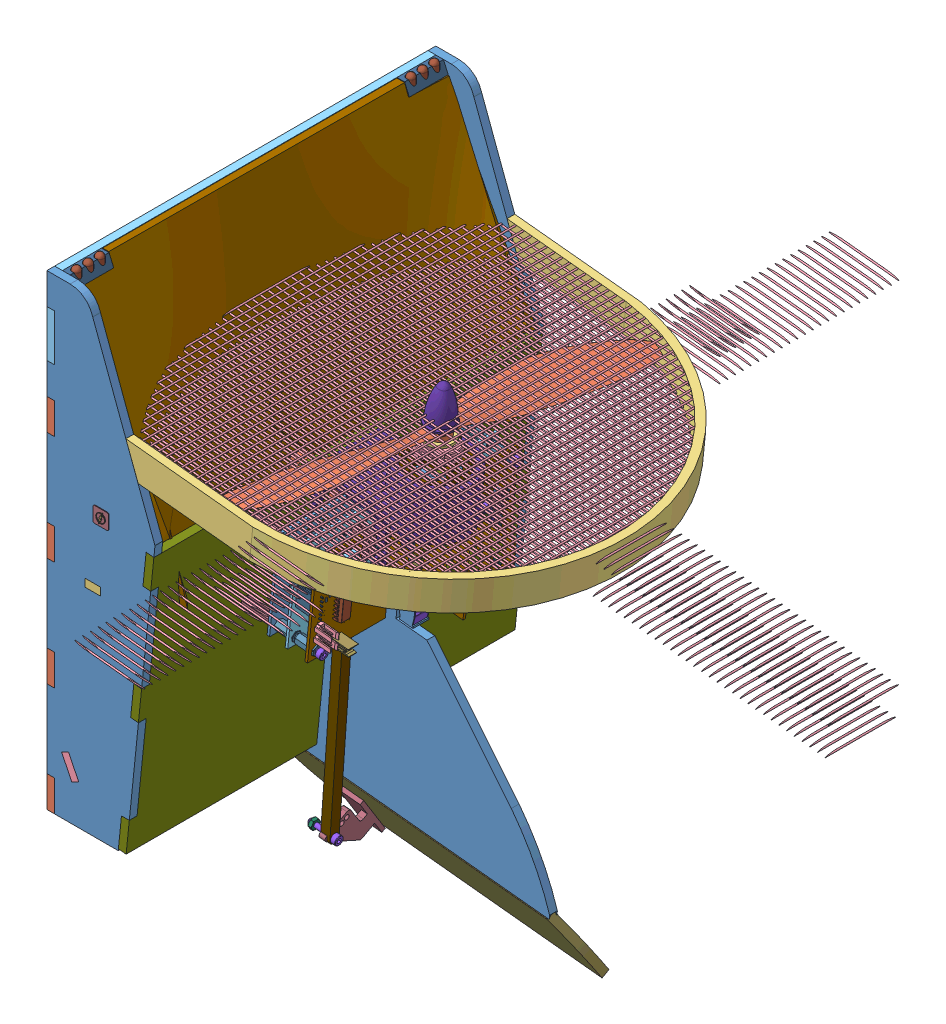
SolidWorks assembly AssTotaleSimu3, configuration Défaut. Lengths in mm. (continued)
Components (placement in the parent): (continued)
- AssStructSimu-1: AssStructSimu [Défaut] at (-125.7658 -1.8483 624.6548) x (1 0 0) z (0 0 -1) size (253.25 324.59 251.6) (continued)
  - AssProtec-1: AssProtec [Défaut] at (86.6746 190.4649 284.6351) x (0 0 -1) z (0.101852 -0.9948 0) size (250 237.46 20) (continued)
    - AssGrillage-2: AssGrillage [Défaut] at (339.6086 -132.5428 241.6839) x (0 0 1) z (-1 0 0) size (2.02 237.05 250) (continued)
      - barreau-208: barreau [Défaut] at (-0.1839 -1.5314 233.7823) x (0.998922 0 0.04641) z (0 1 0) size (1 1 400)
      - barreau-209: barreau [Défaut] at (-0.1839 -1.5314 228.7823) x (0.998922 0 0.04641) z (0 1 0) size (1 1 400)
      - barreau-210: barreau [Défaut] at (-0.1839 -1.5314 223.7823) x (0.998922 0 0.04641) z (0 1 0) size (1 1 400)
      - barreau-211: barreau [Défaut] at (-0.1839 -1.5314 218.7823) x (0.998922 0 0.04641) z (0 1 0) size (1 1 400)
      - barreau-212: barreau [Défaut] at (-0.1839 -1.5314 213.7823) x (0.998922 0 0.04641) z (0 1 0) size (1 1 400)
      - barreau-213: barreau [Défaut] at (-0.1839 -1.5314 208.7823) x (0.998922 0 0.04641) z (0 1 0) size (1 1 400)
      - barreau-214: barreau [Défaut] at (-0.1839 -1.5314 203.7823) x (0.998922 0 0.04641) z (0 1 0) size (1 1 400)
  - AssCarte-1: AssCarte [Défaut] at (38.0121 147.1029 290.772) x (-0.101852 0.9948 0) z (0.9948 0.101852 0) size (66.52 130.57 98.72)
    - carte_onduleur_v3-1: carte_onduleur_v3 [Défaut] at (-131.8199 12.0892 20.7912) size (66.52 130.57 82.34)
      - Layer_1-1: Layer_1 [Défaut] at origin size (60 130 1.61)
      - BTN-1: BTN [Défaut] at (-25.5 7.4 0.803) x (0 -1 0) z (0 0 1) size (6.76 3.64 4.37)
        - Open CASCADE STEP translator 6.8 1.2.1-1: Open CASCADE STEP translator 6.8 1.2.1 [Défaut] at origin size (6.76 3.64 4.37)
          - Body_1-1: Body_1 [Défaut] at (-0.5 -2 0) size (6.76 3.64 4.37)
            - =_[0_1_1_3]-1: =_[0_1_1_3] [Défaut] at origin size (6 3.64 4.37)
            - =_[0_1_1_4]-1: =_[0_1_1_4] [Défaut] at origin size (0.38 1 0.67)
            - =_[0_1_1_5]-1: =_[0_1_1_5] [Défaut] at origin size (0.38 1 0.67)
      - CON_IO1-1: CON_IO1 [Défaut] at (-11.3 12.1 0.803) x (0 -1 0) z (0 0 1) size (13 30 57.5)
        - Open CASCADE STEP translator 6.8 1.3.1-1: Open CASCADE STEP translator 6.8 1.3.1 [Défaut] at origin size (13 30 57.5)
          - Body_1_2-1: Body_1_2 [Défaut] at (-3 -15 8) x (0 -1 0) z (-1 0 0) size (30 57.5 13)
            - 1-1: 1 [Défaut] at origin size (30 50 1.61)
            - 10-1: 10 [Défaut] at (-14.395 31.0465 0.803) x (-1 0 0) z (0 0 1) size (5.59 6.35 1.11)
              - =_[0_1_1_4]-1: =_[0_1_1_4] [Défaut] at origin size (5.59 6.35 1.11)
                - 11-1: 11 [Défaut] at (2 3.3 0) x (-1 0 0) z (0 0 1) size (5.59 6.35 1.11)
                  - =_[0_1_1_3]_2-1: =_[0_1_1_3]_2 [Défaut] at origin size (0.44 0.55 0.36)
                  - =_[0_1_1_4]_2-1: =_[0_1_1_4]_2 [Défaut] at origin size (5.59 4.15 0.36)
                  - =_[0_1_1_5]_2-1: =_[0_1_1_5]_2 [Défaut] at origin size (5.35 6.1 1.1)
                  - =_[0_1_1_6]-1: =_[0_1_1_6] [Défaut] at origin size (0.44 0.55 0.36)
                  - =_[0_1_1_7]-1: =_[0_1_1_7] [Défaut] at origin size (0.44 0.55 0.36)
                  - =_[0_1_1_8]-1: =_[0_1_1_8] [Défaut] at origin size (0.44 0.55 0.36)
            - 13-1: 13 [Défaut] at (-12.62 16.6 -0.803) x (-1 0 0) z (0 0 -1) size (5.59 6.35 1.11)
              - =_[0_1_1_13]-1: =_[0_1_1_13] [Défaut] at origin size (5.59 6.35 1.11)
                - 11-1: 11 [Défaut] at (2 3.3 0) x (-1 0 0) z (0 0 1) size (5.59 6.35 1.11)
                  - =_[0_1_1_3]_2-1: =_[0_1_1_3]_2 [Défaut] at origin size (0.44 0.55 0.36)
                  - =_[0_1_1_4]_2-1: =_[0_1_1_4]_2 [Défaut] at origin size (5.59 4.15 0.36)
                  - =_[0_1_1_5]_2-1: =_[0_1_1_5]_2 [Défaut] at origin size (5.35 6.1 1.1)
                  - =_[0_1_1_6]-1: =_[0_1_1_6] [Défaut] at origin size (0.44 0.55 0.36)
                  - =_[0_1_1_7]-1: =_[0_1_1_7] [Défaut] at origin size (0.44 0.55 0.36)
                  - =_[0_1_1_8]-1: =_[0_1_1_8] [Défaut] at origin size (0.44 0.55 0.36)
            - 16-1: 16 [Défaut] at (-4.2 24.2 0.803) x (-1 0 0) z (0 0 1) size (12.8 0.5 13)
              - =_[0_1_1_15]-1: =_[0_1_1_15] [Défaut] at origin size (12.8 0.5 13)
                - 17-1: 17 [Défaut] at (2.7 0 0) x (1 0 0) z (0 -1 0) size (12.8 13 0.5)
            - 19-1: 19 [Défaut] at (-4.1 6.8 0.803) x (-1 0 0) z (0 0 1) size (12.8 0.5 13)
              - =_[0_1_1_18]-1: =_[0_1_1_18] [Défaut] at origin size (12.8 0.5 13)
                - 17-1: 17 [Défaut] at (2.7 0 0) x (1 0 0) z (0 -1 0) size (12.8 13 0.5)
            - 24-1: 24 [Défaut] at (-8.1 16.5 -0.803) x (0 1 0) z (0 0 -1) size (7.75 5.13 1.17)
              - =_[0_1_1_20]-1: =_[0_1_1_20] [Défaut] at origin size (7.75 5.13 1.17)
                - 20-1: 20 [Défaut] at origin size (7.59 5.13 1.07)
                - 21-1: 21 [Défaut] at (-14.478 0 0) x (-1 0 0) z (0 0 1) size (0.76 5.08 1.17)
                - 22-1: 22 [Défaut] at origin size (0.76 5.08 1.17)
            - 35-1: 35 [Défaut] at (-25.3 25.5 0.803) x (0 -1 0) z (0 0 1) size (6.05 5.2 1.7)
              - =_[0_1_1_25]-1: =_[0_1_1_25] [Défaut] at origin size (6.05 5.2 1.7)
                - 25-1: 25 [Défaut] at origin size (4.3 5.2 1.53)
                - 26-1: 26 [Défaut] at origin size (0.88 0.51 1.06)
                - 27-1: 27 [Défaut] at origin size (0.88 0.51 1.06)
                - 28-1: 28 [Défaut] at origin size (0.88 0.51 1.06)
                - 29-1: 29 [Défaut] at origin size (0.88 0.51 1.06)
                - 30-1: 30 [Défaut] at (11.6 -5.08 0) x (-1 0 0) z (0 0 1) size (0.87 0.51 1.06)
                - 31-1: 31 [Défaut] at (11.6 -2.54 0) x (-1 0 0) z (0 0 1) size (0.87 0.51 1.06)
                - 32-1: 32 [Défaut] at (11.6 0 0) x (-1 0 0) z (0 0 1) size (0.87 0.51 1.06)
                - 33-1: 33 [Défaut] at (11.6 2.54 0) x (-1 0 0) z (0 0 1) size (0.87 0.51 1.06)
            - 40-1: 40 [Défaut] at (-27.6 27.2 0.803) size (2.34 1.04 0.5)
              - =_[0_1_1_36]-1: =_[0_1_1_36] [Défaut] at origin size (2.34 1.04 0.5)
                - 36-1: 36 [Défaut] at origin size (2.29 1.04 0.43)
                - 37-1: 37 [Défaut] at (0.3048 0 0) x (-1 0 0) z (0 0 1) size (0.51 1.02 0.5)
                - 38-1: 38 [Défaut] at origin size (0.51 1.02 0.5)
            - 42-1: 42 [Défaut] at (-22.1 21.6 0.803) x (0 1 0) z (0 0 1) size (2.34 1.04 0.5)
              - =_[0_1_1_36]-1: =_[0_1_1_36] [Défaut] at origin size (2.34 1.04 0.5)
                - 36-1: 36 [Défaut] at origin size (2.29 1.04 0.43)
                - 37-1: 37 [Défaut] at (0.3048 0 0) x (-1 0 0) z (0 0 1) size (0.51 1.02 0.5)
                - 38-1: 38 [Défaut] at origin size (0.51 1.02 0.5)
            - 47-1: 47 [Défaut] at (-14.7664 14.5 -0.803) x (-1 0 0) z (0 0 -1) size (2.34 1.04 0.5)
              - =_[0_1_1_42]-1: =_[0_1_1_42] [Défaut] at origin size (2.34 1.04 0.5)
                - 43-1: 43 [Défaut] at origin size (2.29 1.04 0.43)
                - 44-1: 44 [Défaut] at (0.3048 0 0) x (-1 0 0) z (0 0 1) size (0.51 1.02 0.5)
                - 45-1: 45 [Défaut] at origin size (0.51 1.02 0.5)
            - 57-1: 57 [Défaut] at (-15.3 2.7 -0.803) x (0 -1 0) z (0 0 -1) size (10.36 15.24 6.14)
              - =_[0_1_1_47]-1: =_[0_1_1_47] [Défaut] at origin size (10.36 15.24 6.14)
                - 55-1: 55 [Défaut] at (1.8 -1.2 3) x (1 0 0) z (0 1 0) size (10.36 6.14 15.24)
                  - 54-1: 54 [Défaut] at origin size (10.36 6.14 7.62)
                    - 52-1: 52 [Défaut] at origin size (10.36 6.14 2.54)
                      - 48-1: 48 [Défaut] at origin size (8.4 2.54 2.54)
                      - 49-1: 49 [Défaut] at (-0.0461 1.2682 1.27) x (0 0 -1) z (0.999998 -0.002105 0) size (1.95 5.07 7.58)
                    - 52-2: 52 [Défaut] at (0 0 -2.54) size (10.36 6.14 2.54)
                      - 48-1: 48 [Défaut] at origin size (8.4 2.54 2.54)
                      - 49-1: 49 [Défaut] at (-0.0461 1.2682 1.27) x (0 0 -1) z (0.999998 -0.002105 0) size (1.95 5.07 7.58)
                    - 52-3: 52 [Défaut] at (0 0 -5.08) size (10.36 6.14 2.54)
                      - 48-1: 48 [Défaut] at origin size (8.4 2.54 2.54)
                      - 49-1: 49 [Défaut] at (-0.0461 1.2682 1.27) x (0 0 -1) z (0.999998 -0.002105 0) size (1.95 5.07 7.58)
                  - 54-2: 54 [Défaut] at (0 0 -7.62) size (10.36 6.14 7.62)
                    - 52-1: 52 [Défaut] at origin size (10.36 6.14 2.54)
                      - 48-1: 48 [Défaut] at origin size (8.4 2.54 2.54)
                      - 49-1: 49 [Défaut] at (-0.0461 1.2682 1.27) x (0 0 -1) z (0.999998 -0.002105 0) size (1.95 5.07 7.58)
                    - 52-2: 52 [Défaut] at (0 0 -2.54) size (10.36 6.14 2.54)
                      - 48-1: 48 [Défaut] at origin size (8.4 2.54 2.54)
                      - 49-1: 49 [Défaut] at (-0.0461 1.2682 1.27) x (0 0 -1) z (0.999998 -0.002105 0) size (1.95 5.07 7.58)
                    - 52-3: 52 [Défaut] at (0 0 -5.08) size (10.36 6.14 2.54)
                      - 48-1: 48 [Défaut] at origin size (8.4 2.54 2.54)
                      - 49-1: 49 [Défaut] at (-0.0461 1.2682 1.27) x (0 0 -1) z (0.999998 -0.002105 0) size (1.95 5.07 7.58)
            - 59-1: 59 [Défaut] at (-26.5 31 0.803) x (0 -1 0) z (0 0 1) size (2.34 1.04 0.5)
              - =_[0_1_1_42]-1: =_[0_1_1_42] [Défaut] at origin size (2.34 1.04 0.5)
                - 43-1: 43 [Défaut] at origin size (2.29 1.04 0.43)
                - 44-1: 44 [Défaut] at (0.3048 0 0) x (-1 0 0) z (0 0 1) size (0.51 1.02 0.5)
                - 45-1: 45 [Défaut] at origin size (0.51 1.02 0.5)
            - 61-1: 61 [Défaut] at (-21.6 17.8 0.803) x (-1 0 0) z (0 0 1) size (2.34 1.04 0.5)
              - =_[0_1_1_42]-1: =_[0_1_1_42] [Défaut] at origin size (2.34 1.04 0.5)
                - 43-1: 43 [Défaut] at origin size (2.29 1.04 0.43)
                - 44-1: 44 [Défaut] at (0.3048 0 0) x (-1 0 0) z (0 0 1) size (0.51 1.02 0.5)
                - 45-1: 45 [Défaut] at origin size (0.51 1.02 0.5)
            - 74-1: 74 [Défaut] at (-4.9 41.8 0.803) x (0 -1 0) z (0 0 1) size (6 4.9 1.75)
              - =_[0_1_1_56]-1: =_[0_1_1_56] [Défaut] at origin size (6 4.9 1.75)
                - 72-1: 72 [Défaut] at origin size (6 4.9 1.75)
                  - =_[0_1_1_2]-1: =_[0_1_1_2] [Défaut] at origin size (3.9 4.9 1.57)
                  - =_[0_1_1_3]-1: =_[0_1_1_3] [Défaut] at origin size (6 4.22 1)
                    - =_[0_1_1_60]-1: =_[0_1_1_60] [Défaut] at origin size (1.05 0.41 1)
                    - =_[0_1_1_61]-1: =_[0_1_1_61] [Défaut] at origin size (1.05 0.41 1)
                    - =_[0_1_1_62]-1: =_[0_1_1_62] [Défaut] at origin size (1.05 0.41 1)
                    - =_[0_1_1_63]-1: =_[0_1_1_63] [Défaut] at origin size (1.05 0.41 1)
                    - =_[0_1_1_64]-1: =_[0_1_1_64] [Défaut] at origin size (1.05 0.41 1)
                    - =_[0_1_1_65]-1: =_[0_1_1_65] [Défaut] at origin size (1.05 0.41 1)
                    - =_[0_1_1_66]-1: =_[0_1_1_66] [Défaut] at origin size (1.05 0.41 1)
                    - =_[0_1_1_67]-1: =_[0_1_1_67] [Défaut] at origin size (1.05 0.41 1)
            - 76-1: 76 [Défaut] at (-8.5 40.5664 0.803) x (0 1 0) z (0 0 1) size (2.34 1.04 0.5)
              - =_[0_1_1_42]-1: =_[0_1_1_42] [Défaut] at origin size (2.34 1.04 0.5)
                - 43-1: 43 [Défaut] at origin size (2.29 1.04 0.43)
                - 44-1: 44 [Défaut] at (0.3048 0 0) x (-1 0 0) z (0 0 1) size (0.51 1.02 0.5)
                - 45-1: 45 [Défaut] at origin size (0.51 1.02 0.5)
            - 78-1: 78 [Défaut] at (-5.9 46.4 0.803) x (-1 0 0) z (0 0 1) size (2.34 1.04 0.5)
              - =_[0_1_1_42]-1: =_[0_1_1_42] [Défaut] at origin size (2.34 1.04 0.5)
                - 43-1: 43 [Défaut] at origin size (2.29 1.04 0.43)
                - 44-1: 44 [Défaut] at (0.3048 0 0) x (-1 0 0) z (0 0 1) size (0.51 1.02 0.5)
                - 45-1: 45 [Défaut] at origin size (0.51 1.02 0.5)
            - 80-1: 80 [Défaut] at (-7 48.1 0.803) size (2.34 1.04 0.5)
              - =_[0_1_1_42]-1: =_[0_1_1_42] [Défaut] at origin size (2.34 1.04 0.5)
                - 43-1: 43 [Défaut] at origin size (2.29 1.04 0.43)
                - 44-1: 44 [Défaut] at (0.3048 0 0) x (-1 0 0) z (0 0 1) size (0.51 1.02 0.5)
                - 45-1: 45 [Défaut] at origin size (0.51 1.02 0.5)
            - 82-1: 82 [Défaut] at (-6 37.1 0.803) size (2.34 1.04 0.5)
              - =_[0_1_1_42]-1: =_[0_1_1_42] [Défaut] at origin size (2.34 1.04 0.5)
                - 43-1: 43 [Défaut] at origin size (2.29 1.04 0.43)
                - 44-1: 44 [Défaut] at (0.3048 0 0) x (-1 0 0) z (0 0 1) size (0.51 1.02 0.5)
                - 45-1: 45 [Défaut] at origin size (0.51 1.02 0.5)
      - CON_IO2-1: CON_IO2 [Défaut] at (-11.3 -2.7 0.803) x (0 -1 0) z (0 0 1) size (13 30 57.5)
        - Open CASCADE STEP translator 6.8 1.4.1-1: Open CASCADE STEP translator 6.8 1.4.1 [Défaut] at origin size (13 30 57.5)
          - Body_1_2-1: Body_1_2 [Défaut] at (-3 -15 8) x (0 -1 0) z (-1 0 0) size (30 57.5 13)
            - 1-1: 1 [Défaut] at origin size (30 50 1.61)
            - 10-1: 10 [Défaut] at (-14.395 31.0465 0.803) x (-1 0 0) z (0 0 1) size (5.59 6.35 1.11)
              - =_[0_1_1_4]-1: =_[0_1_1_4] [Défaut] at origin size (5.59 6.35 1.11)
                - 11-1: 11 [Défaut] at (2 3.3 0) x (-1 0 0) z (0 0 1) size (5.59 6.35 1.11)
                  - =_[0_1_1_3]_2-1: =_[0_1_1_3]_2 [Défaut] at origin size (0.44 0.55 0.36)
                  - =_[0_1_1_4]_2-1: =_[0_1_1_4]_2 [Défaut] at origin size (5.59 4.15 0.36)
                  - =_[0_1_1_5]_2-1: =_[0_1_1_5]_2 [Défaut] at origin size (5.35 6.1 1.1)
                  - =_[0_1_1_6]-1: =_[0_1_1_6] [Défaut] at origin size (0.44 0.55 0.36)
                  - =_[0_1_1_7]-1: =_[0_1_1_7] [Défaut] at origin size (0.44 0.55 0.36)
                  - =_[0_1_1_8]-1: =_[0_1_1_8] [Défaut] at origin size (0.44 0.55 0.36)
            - 13-1: 13 [Défaut] at (-12.62 16.6 -0.803) x (-1 0 0) z (0 0 -1) size (5.59 6.35 1.11)
              - =_[0_1_1_13]-1: =_[0_1_1_13] [Défaut] at origin size (5.59 6.35 1.11)
                - 11-1: 11 [Défaut] at (2 3.3 0) x (-1 0 0) z (0 0 1) size (5.59 6.35 1.11)
                  - =_[0_1_1_3]_2-1: =_[0_1_1_3]_2 [Défaut] at origin size (0.44 0.55 0.36)
                  - =_[0_1_1_4]_2-1: =_[0_1_1_4]_2 [Défaut] at origin size (5.59 4.15 0.36)
                  - =_[0_1_1_5]_2-1: =_[0_1_1_5]_2 [Défaut] at origin size (5.35 6.1 1.1)
                  - =_[0_1_1_6]-1: =_[0_1_1_6] [Défaut] at origin size (0.44 0.55 0.36)
                  - =_[0_1_1_7]-1: =_[0_1_1_7] [Défaut] at origin size (0.44 0.55 0.36)
                  - =_[0_1_1_8]-1: =_[0_1_1_8] [Défaut] at origin size (0.44 0.55 0.36)
            - 16-1: 16 [Défaut] at (-4.2 24.2 0.803) x (-1 0 0) z (0 0 1) size (12.8 0.5 13)
              - =_[0_1_1_15]-1: =_[0_1_1_15] [Défaut] at origin size (12.8 0.5 13)
                - 17-1: 17 [Défaut] at (2.7 0 0) x (1 0 0) z (0 -1 0) size (12.8 13 0.5)
            - 19-1: 19 [Défaut] at (-4.1 6.8 0.803) x (-1 0 0) z (0 0 1) size (12.8 0.5 13)
              - =_[0_1_1_18]-1: =_[0_1_1_18] [Défaut] at origin size (12.8 0.5 13)
                - 17-1: 17 [Défaut] at (2.7 0 0) x (1 0 0) z (0 -1 0) size (12.8 13 0.5)
            - 24-1: 24 [Défaut] at (-8.1 16.5 -0.803) x (0 1 0) z (0 0 -1) size (7.75 5.13 1.17)
              - =_[0_1_1_20]-1: =_[0_1_1_20] [Défaut] at origin size (7.75 5.13 1.17)
                - 20-1: 20 [Défaut] at origin size (7.59 5.13 1.07)
                - 21-1: 21 [Défaut] at (-14.478 0 0) x (-1 0 0) z (0 0 1) size (0.76 5.08 1.17)
                - 22-1: 22 [Défaut] at origin size (0.76 5.08 1.17)
            - 35-1: 35 [Défaut] at (-25.3 25.5 0.803) x (0 -1 0) z (0 0 1) size (6.05 5.2 1.7)
              - =_[0_1_1_25]-1: =_[0_1_1_25] [Défaut] at origin size (6.05 5.2 1.7)
                - 25-1: 25 [Défaut] at origin size (4.3 5.2 1.53)
                - 26-1: 26 [Défaut] at origin size (0.88 0.51 1.06)
                - 27-1: 27 [Défaut] at origin size (0.88 0.51 1.06)
                - 28-1: 28 [Défaut] at origin size (0.88 0.51 1.06)
                - 29-1: 29 [Défaut] at origin size (0.88 0.51 1.06)
                - 30-1: 30 [Défaut] at (11.6 -5.08 0) x (-1 0 0) z (0 0 1) size (0.87 0.51 1.06)
                - 31-1: 31 [Défaut] at (11.6 -2.54 0) x (-1 0 0) z (0 0 1) size (0.87 0.51 1.06)
                - 32-1: 32 [Défaut] at (11.6 0 0) x (-1 0 0) z (0 0 1) size (0.87 0.51 1.06)
                - 33-1: 33 [Défaut] at (11.6 2.54 0) x (-1 0 0) z (0 0 1) size (0.87 0.51 1.06)
            - 40-1: 40 [Défaut] at (-27.6 27.2 0.803) size (2.34 1.04 0.5)
              - =_[0_1_1_36]-1: =_[0_1_1_36] [Défaut] at origin size (2.34 1.04 0.5)
                - 36-1: 36 [Défaut] at origin size (2.29 1.04 0.43)
                - 37-1: 37 [Défaut] at (0.3048 0 0) x (-1 0 0) z (0 0 1) size (0.51 1.02 0.5)
                - 38-1: 38 [Défaut] at origin size (0.51 1.02 0.5)
            - 42-1: 42 [Défaut] at (-22.1 21.6 0.803) x (0 1 0) z (0 0 1) size (2.34 1.04 0.5)
              - =_[0_1_1_36]-1: =_[0_1_1_36] [Défaut] at origin size (2.34 1.04 0.5)
                - 36-1: 36 [Défaut] at origin size (2.29 1.04 0.43)
                - 37-1: 37 [Défaut] at (0.3048 0 0) x (-1 0 0) z (0 0 1) size (0.51 1.02 0.5)
                - 38-1: 38 [Défaut] at origin size (0.51 1.02 0.5)
            - 47-1: 47 [Défaut] at (-14.7664 14.5 -0.803) x (-1 0 0) z (0 0 -1) size (2.34 1.04 0.5)
              - =_[0_1_1_42]-1: =_[0_1_1_42] [Défaut] at origin size (2.34 1.04 0.5)
                - 43-1: 43 [Défaut] at origin size (2.29 1.04 0.43)
                - 44-1: 44 [Défaut] at (0.3048 0 0) x (-1 0 0) z (0 0 1) size (0.51 1.02 0.5)
                - 45-1: 45 [Défaut] at origin size (0.51 1.02 0.5)
            - 57-1: 57 [Défaut] at (-15.3 2.7 -0.803) x (0 -1 0) z (0 0 -1) size (10.36 15.24 6.14)
              - =_[0_1_1_47]-1: =_[0_1_1_47] [Défaut] at origin size (10.36 15.24 6.14)
                - 55-1: 55 [Défaut] at (1.8 -1.2 3) x (1 0 0) z (0 1 0) size (10.36 6.14 15.24)
                  - 54-1: 54 [Défaut] at origin size (10.36 6.14 7.62)
                    - 52-1: 52 [Défaut] at origin size (10.36 6.14 2.54)
                      - 48-1: 48 [Défaut] at origin size (8.4 2.54 2.54)
                      - 49-1: 49 [Défaut] at (-0.0461 1.2682 1.27) x (0 0 -1) z (0.999998 -0.002105 0) size (1.95 5.07 7.58)
                    - 52-2: 52 [Défaut] at (0 0 -2.54) size (10.36 6.14 2.54)
                      - 48-1: 48 [Défaut] at origin size (8.4 2.54 2.54)
                      - 49-1: 49 [Défaut] at (-0.0461 1.2682 1.27) x (0 0 -1) z (0.999998 -0.002105 0) size (1.95 5.07 7.58)
                    - 52-3: 52 [Défaut] at (0 0 -5.08) size (10.36 6.14 2.54)
                      - 48-1: 48 [Défaut] at origin size (8.4 2.54 2.54)
                      - 49-1: 49 [Défaut] at (-0.0461 1.2682 1.27) x (0 0 -1) z (0.999998 -0.002105 0) size (1.95 5.07 7.58)
                  - 54-2: 54 [Défaut] at (0 0 -7.62) size (10.36 6.14 7.62)
                    - 52-1: 52 [Défaut] at origin size (10.36 6.14 2.54)
                      - 48-1: 48 [Défaut] at origin size (8.4 2.54 2.54)
                      - 49-1: 49 [Défaut] at (-0.0461 1.2682 1.27) x (0 0 -1) z (0.999998 -0.002105 0) size (1.95 5.07 7.58)
                    - 52-2: 52 [Défaut] at (0 0 -2.54) size (10.36 6.14 2.54)
                      - 48-1: 48 [Défaut] at origin size (8.4 2.54 2.54)
                      - 49-1: 49 [Défaut] at (-0.0461 1.2682 1.27) x (0 0 -1) z (0.999998 -0.002105 0) size (1.95 5.07 7.58)
                    - 52-3: 52 [Défaut] at (0 0 -5.08) size (10.36 6.14 2.54)
                      - 48-1: 48 [Défaut] at origin size (8.4 2.54 2.54)
                      - 49-1: 49 [Défaut] at (-0.0461 1.2682 1.27) x (0 0 -1) z (0.999998 -0.002105 0) size (1.95 5.07 7.58)
            - 59-1: 59 [Défaut] at (-26.5 31 0.803) x (0 -1 0) z (0 0 1) size (2.34 1.04 0.5)
              - =_[0_1_1_42]-1: =_[0_1_1_42] [Défaut] at origin size (2.34 1.04 0.5)
                - 43-1: 43 [Défaut] at origin size (2.29 1.04 0.43)
                - 44-1: 44 [Défaut] at (0.3048 0 0) x (-1 0 0) z (0 0 1) size (0.51 1.02 0.5)
                - 45-1: 45 [Défaut] at origin size (0.51 1.02 0.5)
            - 61-1: 61 [Défaut] at (-21.6 17.8 0.803) x (-1 0 0) z (0 0 1) size (2.34 1.04 0.5)
              - =_[0_1_1_42]-1: =_[0_1_1_42] [Défaut] at origin size (2.34 1.04 0.5)
                - 43-1: 43 [Défaut] at origin size (2.29 1.04 0.43)
                - 44-1: 44 [Défaut] at (0.3048 0 0) x (-1 0 0) z (0 0 1) size (0.51 1.02 0.5)
                - 45-1: 45 [Défaut] at origin size (0.51 1.02 0.5)
            - 74-1: 74 [Défaut] at (-4.9 41.8 0.803) x (0 -1 0) z (0 0 1) size (6 4.9 1.75)
              - =_[0_1_1_56]-1: =_[0_1_1_56] [Défaut] at origin size (6 4.9 1.75)
                - 72-1: 72 [Défaut] at origin size (6 4.9 1.75)
                  - =_[0_1_1_2]-1: =_[0_1_1_2] [Défaut] at origin size (3.9 4.9 1.57)
                  - =_[0_1_1_3]-1: =_[0_1_1_3] [Défaut] at origin size (6 4.22 1)
                    - =_[0_1_1_60]-1: =_[0_1_1_60] [Défaut] at origin size (1.05 0.41 1)
                    - =_[0_1_1_61]-1: =_[0_1_1_61] [Défaut] at origin size (1.05 0.41 1)
                    - =_[0_1_1_62]-1: =_[0_1_1_62] [Défaut] at origin size (1.05 0.41 1)
                    - =_[0_1_1_63]-1: =_[0_1_1_63] [Défaut] at origin size (1.05 0.41 1)
                    - =_[0_1_1_64]-1: =_[0_1_1_64] [Défaut] at origin size (1.05 0.41 1)
                    - =_[0_1_1_65]-1: =_[0_1_1_65] [Défaut] at origin size (1.05 0.41 1)
                    - =_[0_1_1_66]-1: =_[0_1_1_66] [Défaut] at origin size (1.05 0.41 1)
                    - =_[0_1_1_67]-1: =_[0_1_1_67] [Défaut] at origin size (1.05 0.41 1)
            - 76-1: 76 [Défaut] at (-8.5 40.5664 0.803) x (0 1 0) z (0 0 1) size (2.34 1.04 0.5)
              - =_[0_1_1_42]-1: =_[0_1_1_42] [Défaut] at origin size (2.34 1.04 0.5)
                - 43-1: 43 [Défaut] at origin size (2.29 1.04 0.43)
                - 44-1: 44 [Défaut] at (0.3048 0 0) x (-1 0 0) z (0 0 1) size (0.51 1.02 0.5)
                - 45-1: 45 [Défaut] at origin size (0.51 1.02 0.5)
            - 78-1: 78 [Défaut] at (-5.9 46.4 0.803) x (-1 0 0) z (0 0 1) size (2.34 1.04 0.5)
              - =_[0_1_1_42]-1: =_[0_1_1_42] [Défaut] at origin size (2.34 1.04 0.5)
                - 43-1: 43 [Défaut] at origin size (2.29 1.04 0.43)
                - 44-1: 44 [Défaut] at (0.3048 0 0) x (-1 0 0) z (0 0 1) size (0.51 1.02 0.5)
                - 45-1: 45 [Défaut] at origin size (0.51 1.02 0.5)
            - 80-1: 80 [Défaut] at (-7 48.1 0.803) size (2.34 1.04 0.5)
              - =_[0_1_1_42]-1: =_[0_1_1_42] [Défaut] at origin size (2.34 1.04 0.5)
                - 43-1: 43 [Défaut] at origin size (2.29 1.04 0.43)
                - 44-1: 44 [Défaut] at (0.3048 0 0) x (-1 0 0) z (0 0 1) size (0.51 1.02 0.5)
                - 45-1: 45 [Défaut] at origin size (0.51 1.02 0.5)
            - 82-1: 82 [Défaut] at (-6 37.1 0.803) size (2.34 1.04 0.5)
              - =_[0_1_1_42]-1: =_[0_1_1_42] [Défaut] at origin size (2.34 1.04 0.5)
                - 43-1: 43 [Défaut] at origin size (2.29 1.04 0.43)
                - 44-1: 44 [Défaut] at (0.3048 0 0) x (-1 0 0) z (0 0 1) size (0.51 1.02 0.5)
                - 45-1: 45 [Défaut] at origin size (0.51 1.02 0.5)
      - CON_IO3-1: CON_IO3 [Défaut] at (-11.3 -17.7 0.803) x (0 -1 0) z (0 0 1) size (13 30 57.5)
        - Open CASCADE STEP translator 6.8 1.5.1-1: Open CASCADE STEP translator 6.8 1.5.1 [Défaut] at origin size (13 30 57.5)
          - Body_1_2-1: Body_1_2 [Défaut] at (-3 -15 8) x (0 -1 0) z (-1 0 0) size (30 57.5 13)
            - 1-1: 1 [Défaut] at origin size (30 50 1.61)
            - 10-1: 10 [Défaut] at (-14.395 31.0465 0.803) x (-1 0 0) z (0 0 1) size (5.59 6.35 1.11)
              - =_[0_1_1_4]-1: =_[0_1_1_4] [Défaut] at origin size (5.59 6.35 1.11)
                - 11-1: 11 [Défaut] at (2 3.3 0) x (-1 0 0) z (0 0 1) size (5.59 6.35 1.11)
                  - =_[0_1_1_3]_2-1: =_[0_1_1_3]_2 [Défaut] at origin size (0.44 0.55 0.36)
                  - =_[0_1_1_4]_2-1: =_[0_1_1_4]_2 [Défaut] at origin size (5.59 4.15 0.36)
                  - =_[0_1_1_5]_2-1: =_[0_1_1_5]_2 [Défaut] at origin size (5.35 6.1 1.1)
                  - =_[0_1_1_6]-1: =_[0_1_1_6] [Défaut] at origin size (0.44 0.55 0.36)
                  - =_[0_1_1_7]-1: =_[0_1_1_7] [Défaut] at origin size (0.44 0.55 0.36)
                  - =_[0_1_1_8]-1: =_[0_1_1_8] [Défaut] at origin size (0.44 0.55 0.36)
            - 13-1: 13 [Défaut] at (-12.62 16.6 -0.803) x (-1 0 0) z (0 0 -1) size (5.59 6.35 1.11)
              - =_[0_1_1_13]-1: =_[0_1_1_13] [Défaut] at origin size (5.59 6.35 1.11)
                - 11-1: 11 [Défaut] at (2 3.3 0) x (-1 0 0) z (0 0 1) size (5.59 6.35 1.11)
                  - =_[0_1_1_3]_2-1: =_[0_1_1_3]_2 [Défaut] at origin size (0.44 0.55 0.36)
                  - =_[0_1_1_4]_2-1: =_[0_1_1_4]_2 [Défaut] at origin size (5.59 4.15 0.36)
                  - =_[0_1_1_5]_2-1: =_[0_1_1_5]_2 [Défaut] at origin size (5.35 6.1 1.1)
                  - =_[0_1_1_6]-1: =_[0_1_1_6] [Défaut] at origin size (0.44 0.55 0.36)
                  - =_[0_1_1_7]-1: =_[0_1_1_7] [Défaut] at origin size (0.44 0.55 0.36)
                  - =_[0_1_1_8]-1: =_[0_1_1_8] [Défaut] at origin size (0.44 0.55 0.36)
            - 16-1: 16 [Défaut] at (-4.2 24.2 0.803) x (-1 0 0) z (0 0 1) size (12.8 0.5 13)
              - =_[0_1_1_15]-1: =_[0_1_1_15] [Défaut] at origin size (12.8 0.5 13)
                - 17-1: 17 [Défaut] at (2.7 0 0) x (1 0 0) z (0 -1 0) size (12.8 13 0.5)
            - 19-1: 19 [Défaut] at (-4.1 6.8 0.803) x (-1 0 0) z (0 0 1) size (12.8 0.5 13)
              - =_[0_1_1_18]-1: =_[0_1_1_18] [Défaut] at origin size (12.8 0.5 13)
                - 17-1: 17 [Défaut] at (2.7 0 0) x (1 0 0) z (0 -1 0) size (12.8 13 0.5)
            - 24-1: 24 [Défaut] at (-8.1 16.5 -0.803) x (0 1 0) z (0 0 -1) size (7.75 5.13 1.17)
              - =_[0_1_1_20]-1: =_[0_1_1_20] [Défaut] at origin size (7.75 5.13 1.17)
                - 20-1: 20 [Défaut] at origin size (7.59 5.13 1.07)
                - 21-1: 21 [Défaut] at (-14.478 0 0) x (-1 0 0) z (0 0 1) size (0.76 5.08 1.17)
                - 22-1: 22 [Défaut] at origin size (0.76 5.08 1.17)
            - 35-1: 35 [Défaut] at (-25.3 25.5 0.803) x (0 -1 0) z (0 0 1) size (6.05 5.2 1.7)
              - =_[0_1_1_25]-1: =_[0_1_1_25] [Défaut] at origin size (6.05 5.2 1.7)
                - 25-1: 25 [Défaut] at origin size (4.3 5.2 1.53)
                - 26-1: 26 [Défaut] at origin size (0.88 0.51 1.06)
                - 27-1: 27 [Défaut] at origin size (0.88 0.51 1.06)
                - 28-1: 28 [Défaut] at origin size (0.88 0.51 1.06)
                - 29-1: 29 [Défaut] at origin size (0.88 0.51 1.06)
                - 30-1: 30 [Défaut] at (11.6 -5.08 0) x (-1 0 0) z (0 0 1) size (0.87 0.51 1.06)
                - 31-1: 31 [Défaut] at (11.6 -2.54 0) x (-1 0 0) z (0 0 1) size (0.87 0.51 1.06)
                - 32-1: 32 [Défaut] at (11.6 0 0) x (-1 0 0) z (0 0 1) size (0.87 0.51 1.06)
                - 33-1: 33 [Défaut] at (11.6 2.54 0) x (-1 0 0) z (0 0 1) size (0.87 0.51 1.06)
            - 40-1: 40 [Défaut] at (-27.6 27.2 0.803) size (2.34 1.04 0.5)
              - =_[0_1_1_36]-1: =_[0_1_1_36] [Défaut] at origin size (2.34 1.04 0.5)
                - 36-1: 36 [Défaut] at origin size (2.29 1.04 0.43)
                - 37-1: 37 [Défaut] at (0.3048 0 0) x (-1 0 0) z (0 0 1) size (0.51 1.02 0.5)
                - 38-1: 38 [Défaut] at origin size (0.51 1.02 0.5)
            - 42-1: 42 [Défaut] at (-22.1 21.6 0.803) x (0 1 0) z (0 0 1) size (2.34 1.04 0.5)
              - =_[0_1_1_36]-1: =_[0_1_1_36] [Défaut] at origin size (2.34 1.04 0.5)
                - 36-1: 36 [Défaut] at origin size (2.29 1.04 0.43)
                - 37-1: 37 [Défaut] at (0.3048 0 0) x (-1 0 0) z (0 0 1) size (0.51 1.02 0.5)
                - 38-1: 38 [Défaut] at origin size (0.51 1.02 0.5)
            - 47-1: 47 [Défaut] at (-14.7664 14.5 -0.803) x (-1 0 0) z (0 0 -1) size (2.34 1.04 0.5)
              - =_[0_1_1_42]-1: =_[0_1_1_42] [Défaut] at origin size (2.34 1.04 0.5)
                - 43-1: 43 [Défaut] at origin size (2.29 1.04 0.43)
                - 44-1: 44 [Défaut] at (0.3048 0 0) x (-1 0 0) z (0 0 1) size (0.51 1.02 0.5)
                - 45-1: 45 [Défaut] at origin size (0.51 1.02 0.5)
            - 57-1: 57 [Défaut] at (-15.3 2.7 -0.803) x (0 -1 0) z (0 0 -1) size (10.36 15.24 6.14)
              - =_[0_1_1_47]-1: =_[0_1_1_47] [Défaut] at origin size (10.36 15.24 6.14)
                - 55-1: 55 [Défaut] at (1.8 -1.2 3) x (1 0 0) z (0 1 0) size (10.36 6.14 15.24)
                  - 54-1: 54 [Défaut] at origin size (10.36 6.14 7.62)
                    - 52-1: 52 [Défaut] at origin size (10.36 6.14 2.54)
                      - 48-1: 48 [Défaut] at origin size (8.4 2.54 2.54)
                      - 49-1: 49 [Défaut] at (-0.0461 1.2682 1.27) x (0 0 -1) z (0.999998 -0.002105 0) size (1.95 5.07 7.58)
                    - 52-2: 52 [Défaut] at (0 0 -2.54) size (10.36 6.14 2.54)
                      - 48-1: 48 [Défaut] at origin size (8.4 2.54 2.54)
                      - 49-1: 49 [Défaut] at (-0.0461 1.2682 1.27) x (0 0 -1) z (0.999998 -0.002105 0) size (1.95 5.07 7.58)
                    - 52-3: 52 [Défaut] at (0 0 -5.08) size (10.36 6.14 2.54)
                      - 48-1: 48 [Défaut] at origin size (8.4 2.54 2.54)
                      - 49-1: 49 [Défaut] at (-0.0461 1.2682 1.27) x (0 0 -1) z (0.999998 -0.002105 0) size (1.95 5.07 7.58)
                  - 54-2: 54 [Défaut] at (0 0 -7.62) size (10.36 6.14 7.62)
                    - 52-1: 52 [Défaut] at origin size (10.36 6.14 2.54)
                      - 48-1: 48 [Défaut] at origin size (8.4 2.54 2.54)
                      - 49-1: 49 [Défaut] at (-0.0461 1.2682 1.27) x (0 0 -1) z (0.999998 -0.002105 0) size (1.95 5.07 7.58)
                    - 52-2: 52 [Défaut] at (0 0 -2.54) size (10.36 6.14 2.54)
                      - 48-1: 48 [Défaut] at origin size (8.4 2.54 2.54)
                      - 49-1: 49 [Défaut] at (-0.0461 1.2682 1.27) x (0 0 -1) z (0.999998 -0.002105 0) size (1.95 5.07 7.58)
                    - 52-3: 52 [Défaut] at (0 0 -5.08) size (10.36 6.14 2.54)
                      - 48-1: 48 [Défaut] at origin size (8.4 2.54 2.54)
                      - 49-1: 49 [Défaut] at (-0.0461 1.2682 1.27) x (0 0 -1) z (0.999998 -0.002105 0) size (1.95 5.07 7.58)
            - 59-1: 59 [Défaut] at (-26.5 31 0.803) x (0 -1 0) z (0 0 1) size (2.34 1.04 0.5)
              - =_[0_1_1_42]-1: =_[0_1_1_42] [Défaut] at origin size (2.34 1.04 0.5)
                - 43-1: 43 [Défaut] at origin size (2.29 1.04 0.43)
                - 44-1: 44 [Défaut] at (0.3048 0 0) x (-1 0 0) z (0 0 1) size (0.51 1.02 0.5)
                - 45-1: 45 [Défaut] at origin size (0.51 1.02 0.5)
            - 61-1: 61 [Défaut] at (-21.6 17.8 0.803) x (-1 0 0) z (0 0 1) size (2.34 1.04 0.5)
              - =_[0_1_1_42]-1: =_[0_1_1_42] [Défaut] at origin size (2.34 1.04 0.5)
                - 43-1: 43 [Défaut] at origin size (2.29 1.04 0.43)
                - 44-1: 44 [Défaut] at (0.3048 0 0) x (-1 0 0) z (0 0 1) size (0.51 1.02 0.5)
                - 45-1: 45 [Défaut] at origin size (0.51 1.02 0.5)
            - 74-1: 74 [Défaut] at (-4.9 41.8 0.803) x (0 -1 0) z (0 0 1) size (6 4.9 1.75)
              - =_[0_1_1_56]-1: =_[0_1_1_56] [Défaut] at origin size (6 4.9 1.75)
                - 72-1: 72 [Défaut] at origin size (6 4.9 1.75)
                  - =_[0_1_1_2]-1: =_[0_1_1_2] [Défaut] at origin size (3.9 4.9 1.57)
                  - =_[0_1_1_3]-1: =_[0_1_1_3] [Défaut] at origin size (6 4.22 1)
                    - =_[0_1_1_60]-1: =_[0_1_1_60] [Défaut] at origin size (1.05 0.41 1)
                    - =_[0_1_1_61]-1: =_[0_1_1_61] [Défaut] at origin size (1.05 0.41 1)
                    - =_[0_1_1_62]-1: =_[0_1_1_62] [Défaut] at origin size (1.05 0.41 1)
                    - =_[0_1_1_63]-1: =_[0_1_1_63] [Défaut] at origin size (1.05 0.41 1)
                    - =_[0_1_1_64]-1: =_[0_1_1_64] [Défaut] at origin size (1.05 0.41 1)
                    - =_[0_1_1_65]-1: =_[0_1_1_65] [Défaut] at origin size (1.05 0.41 1)
                    - =_[0_1_1_66]-1: =_[0_1_1_66] [Défaut] at origin size (1.05 0.41 1)
                    - =_[0_1_1_67]-1: =_[0_1_1_67] [Défaut] at origin size (1.05 0.41 1)
            - 76-1: 76 [Défaut] at (-8.5 40.5664 0.803) x (0 1 0) z (0 0 1) size (2.34 1.04 0.5)
              - =_[0_1_1_42]-1: =_[0_1_1_42] [Défaut] at origin size (2.34 1.04 0.5)
                - 43-1: 43 [Défaut] at origin size (2.29 1.04 0.43)
                - 44-1: 44 [Défaut] at (0.3048 0 0) x (-1 0 0) z (0 0 1) size (0.51 1.02 0.5)
                - 45-1: 45 [Défaut] at origin size (0.51 1.02 0.5)
            - 78-1: 78 [Défaut] at (-5.9 46.4 0.803) x (-1 0 0) z (0 0 1) size (2.34 1.04 0.5)
              - =_[0_1_1_42]-1: =_[0_1_1_42] [Défaut] at origin size (2.34 1.04 0.5)
                - 43-1: 43 [Défaut] at origin size (2.29 1.04 0.43)
                - 44-1: 44 [Défaut] at (0.3048 0 0) x (-1 0 0) z (0 0 1) size (0.51 1.02 0.5)
                - 45-1: 45 [Défaut] at origin size (0.51 1.02 0.5)
            - 80-1: 80 [Défaut] at (-7 48.1 0.803) size (2.34 1.04 0.5)
              - =_[0_1_1_42]-1: =_[0_1_1_42] [Défaut] at origin size (2.34 1.04 0.5)
                - 43-1: 43 [Défaut] at origin size (2.29 1.04 0.43)
                - 44-1: 44 [Défaut] at (0.3048 0 0) x (-1 0 0) z (0 0 1) size (0.51 1.02 0.5)
                - 45-1: 45 [Défaut] at origin size (0.51 1.02 0.5)
            - 82-1: 82 [Défaut] at (-6 37.1 0.803) size (2.34 1.04 0.5)
              - =_[0_1_1_42]-1: =_[0_1_1_42] [Défaut] at origin size (2.34 1.04 0.5)
                - 43-1: 43 [Défaut] at origin size (2.29 1.04 0.43)
                - 44-1: 44 [Défaut] at (0.3048 0 0) x (-1 0 0) z (0 0 1) size (0.51 1.02 0.5)
                - 45-1: 45 [Défaut] at origin size (0.51 1.02 0.5)
      - C1_1-1: C1_1 [Défaut] at (-20.6336 6.4 -0.803) x (1 0 0) z (0 0 -1) size (2.34 1.04 0.5)
        - Open CASCADE STEP translator 6.8 1.6.1-1: Open CASCADE STEP translator 6.8 1.6.1 [Défaut] at origin size (2.34 1.04 0.5)
          - Body_1-1: Body_1 [Défaut] at origin size (2.29 1.04 0.43)
          - Pin_1-1: Pin_1 [Défaut] at (0.3048 0 0) x (-1 0 0) z (0 0 1) size (0.51 1.02 0.5)
          - Pin_2-1: Pin_2 [Défaut] at origin size (0.51 1.02 0.5)
      - C1_2-1: C1_2 [Défaut] at (-24.2 6.4 -0.803) x (1 0 0) z (0 0 -1) size (2.34 1.04 0.5)
        - Open CASCADE STEP translator 6.8 1.6.1-1: Open CASCADE STEP translator 6.8 1.6.1 [Défaut] at origin size (2.34 1.04 0.5)
          - Body_1-1: Body_1 [Défaut] at origin size (2.29 1.04 0.43)
          - Pin_1-1: Pin_1 [Défaut] at (0.3048 0 0) x (-1 0 0) z (0 0 1) size (0.51 1.02 0.5)
          - Pin_2-1: Pin_2 [Défaut] at origin size (0.51 1.02 0.5)
      - C_F-1: C_F [Défaut] at (-16.2432 4.45 -0.803) x (0 -1 0) z (0 0 -1) size (2.34 1.04 0.5)
        - Open CASCADE STEP translator 6.8 1.6.1-1: Open CASCADE STEP translator 6.8 1.6.1 [Défaut] at origin size (2.34 1.04 0.5)
          - Body_1-1: Body_1 [Défaut] at origin size (2.29 1.04 0.43)
          - Pin_1-1: Pin_1 [Défaut] at (0.3048 0 0) x (-1 0 0) z (0 0 1) size (0.51 1.02 0.5)
          - Pin_2-1: Pin_2 [Défaut] at origin size (0.51 1.02 0.5)
      - D_LED_STATE1-1: D_LED_STATE1 [Défaut] at (-6.8906 -21.6 0.803) size (2.34 1.04 0.5)
        - Open CASCADE STEP translator 6.8 1.6.1-1: Open CASCADE STEP translator 6.8 1.6.1 [Défaut] at origin size (2.34 1.04 0.5)
          - Body_1-1: Body_1 [Défaut] at origin size (2.29 1.04 0.43)
          - Pin_1-1: Pin_1 [Défaut] at (0.3048 0 0) x (-1 0 0) z (0 0 1) size (0.51 1.02 0.5)
          - Pin_2-1: Pin_2 [Défaut] at origin size (0.51 1.02 0.5)
      - PICKIT-1: PICKIT [Défaut] at (-24.1 -30.5 0.803) size (15.24 5 14.3)
        - Open CASCADE STEP translator 6.8 1.10.1-1: Open CASCADE STEP translator 6.8 1.10.1 [Défaut] at origin size (15.24 5 14.3)
          - Body_1_2-1: Body_1_2 [Défaut] at (6.3 0 12) size (15.24 5 14.3)
      - C_DEC_CUR-1: C_DEC_CUR [Défaut] at (-8.9496 5.7572 -0.803) x (0 1 0) z (0 0 -1) size (2.34 1.04 0.5)
        - Open CASCADE STEP translator 6.8 1.6.1-1: Open CASCADE STEP translator 6.8 1.6.1 [Défaut] at origin size (2.34 1.04 0.5)
          - Body_1-1: Body_1 [Défaut] at origin size (2.29 1.04 0.43)
          - Pin_1-1: Pin_1 [Défaut] at (0.3048 0 0) x (-1 0 0) z (0 0 1) size (0.51 1.02 0.5)
          - Pin_2-1: Pin_2 [Défaut] at origin size (0.51 1.02 0.5)
      - R_F-1: R_F [Défaut] at (-14.65 4.4432 -0.803) x (0 -1 0) z (0 0 -1) size (2.34 1.04 0.5)
        - Open CASCADE STEP translator 6.8 1.12.1-1: Open CASCADE STEP translator 6.8 1.12.1 [Défaut] at origin size (2.34 1.04 0.5)
          - Body_1_3-1: Body_1_3 [Défaut] at origin size (2.29 1.04 0.43)
          - Pin_1_2-1: Pin_1_2 [Défaut] at (0.3048 0 0) x (-1 0 0) z (0 0 1) size (0.51 1.02 0.5)
          - Pin_2_2-1: Pin_2_2 [Défaut] at origin size (0.51 1.02 0.5)
      - R_GAIN1-1: R_GAIN1 [Défaut] at (-13.95 5.7568 -0.803) x (0 1 0) z (0 0 -1) size (2.34 1.04 0.5)
        - Open CASCADE STEP translator 6.8 1.12.1-1: Open CASCADE STEP translator 6.8 1.12.1 [Défaut] at origin size (2.34 1.04 0.5)
          - Body_1_3-1: Body_1_3 [Défaut] at origin size (2.29 1.04 0.43)
          - Pin_1_2-1: Pin_1_2 [Défaut] at (0.3048 0 0) x (-1 0 0) z (0 0 1) size (0.51 1.02 0.5)
          - Pin_2_2-1: Pin_2_2 [Défaut] at origin size (0.51 1.02 0.5)
      - R_GAIN2-1: R_GAIN2 [Défaut] at (-15.65 7.9176 -0.803) x (0 -1 0) z (0 0 -1) size (2.34 1.04 0.5)
        - Open CASCADE STEP translator 6.8 1.12.1-1: Open CASCADE STEP translator 6.8 1.12.1 [Défaut] at origin size (2.34 1.04 0.5)
          - Body_1_3-1: Body_1_3 [Défaut] at origin size (2.29 1.04 0.43)
          - Pin_1_2-1: Pin_1_2 [Défaut] at (0.3048 0 0) x (-1 0 0) z (0 0 1) size (0.51 1.02 0.5)
          - Pin_2_2-1: Pin_2_2 [Défaut] at origin size (0.51 1.02 0.5)
      - R_LED_STATE1-1: R_LED_STATE1 [Défaut] at (-6.9242 -19.9 0.803) size (2.34 1.04 0.5)
        - Open CASCADE STEP translator 6.8 1.12.1-1: Open CASCADE STEP translator 6.8 1.12.1 [Défaut] at origin size (2.34 1.04 0.5)
          - Body_1_3-1: Body_1_3 [Défaut] at origin size (2.29 1.04 0.43)
          - Pin_1_2-1: Pin_1_2 [Défaut] at (0.3048 0 0) x (-1 0 0) z (0 0 1) size (0.51 1.02 0.5)
          - Pin_2_2-1: Pin_2_2 [Défaut] at origin size (0.51 1.02 0.5)
      - R_RESET1-1: R_RESET1 [Défaut] at (-23 7.9 0.803) size (2.34 1.04 0.5)
        - Open CASCADE STEP translator 6.8 1.12.1-1: Open CASCADE STEP translator 6.8 1.12.1 [Défaut] at origin size (2.34 1.04 0.5)
          - Body_1_3-1: Body_1_3 [Défaut] at origin size (2.29 1.04 0.43)
          - Pin_1_2-1: Pin_1_2 [Défaut] at (0.3048 0 0) x (-1 0 0) z (0 0 1) size (0.51 1.02 0.5)
          - Pin_2_2-1: Pin_2_2 [Défaut] at origin size (0.51 1.02 0.5)
